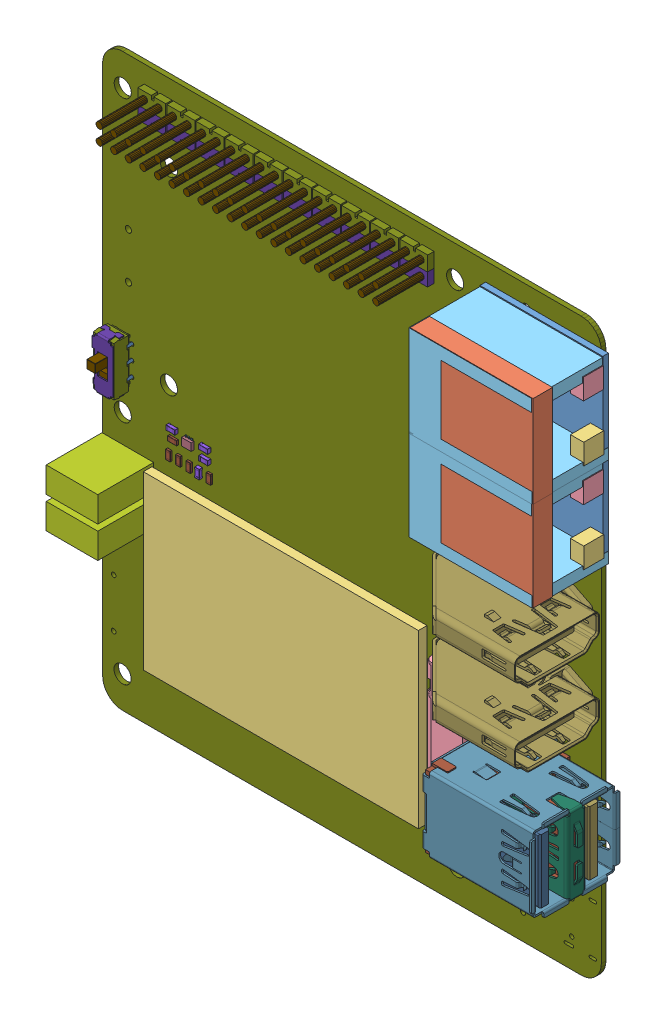
SolidWorks assembly CM4-DUAL-ETH-4G 5G-BASE, configuration Default. Lengths in mm. (continued)
Components (placement in the parent): (continued)
- CM4-DUAL-ETH-4G 5G-BASE.step-1: CM4-DUAL-ETH-4G 5G-BASE.step [Default] at origin size (91.94 99.62 20.53) (continued)
  - C51.step-1: C51.step [Default] at origin size (0.8 1.6 0.6)
    - CAPC1608(0603).step-1: CAPC1608(0603).step [Default] at (59.9278 -41.4202 -0.7984) x (0 1 0) z (0 0 -1) size (1.6 0.8 0.6)
  - C50.step-1: C50.step [Default] at origin size (1.6 0.8 0.6)
    - CAPC1608(0603).step-1: CAPC1608(0603).step [Default] at (29.923 -76.9062 0) x (1 0 0) z (0 0 1) size (1.6 0.8 0.6)
  - C49.step-1: C49.step [Default] at origin size (0.8 1.6 0.6)
    - CAPC1608(0603).step-1: CAPC1608(0603).step [Default] at (38.0407 -61.99 0) x (0 -1 0) z (0 0 1) size (1.6 0.8 0.6)
  - C48.step-1: C48.step [Default] at origin size (1.6 0.8 0.6)
    - CAPC1608(0603).step-1: CAPC1608(0603).step [Default] at (49.0658 -69.8064 0) x (-1 0 0) z (0 0 1) size (1.6 0.8 0.6)
  - C47.step-1: C47.step [Default] at origin size (0.8 1.6 0.6)
    - CAPC1608(0603).step-1: CAPC1608(0603).step [Default] at (39.4963 -61.99 0) x (0 -1 0) z (0 0 1) size (1.6 0.8 0.6)
  - C46.step-1: C46.step [Default] at origin size (1.6 0.8 0.6)
    - CAPC1608(0603).step-1: CAPC1608(0603).step [Default] at (49.0658 -71.2537 0) x (-1 0 0) z (0 0 1) size (1.6 0.8 0.6)
  - C44.step-1: C44.step [Default] at origin size (0.8 1.6 0.6)
    - CAPC1608(0603).step-1: CAPC1608(0603).step [Default] at (42.5195 -81.9688 -0.7984) x (0 1 0) z (0 0 -1) size (1.6 0.8 0.6)
  - C43.step-1: C43.step [Default] at origin size (1.6 0.8 0.6)
    - CAPC1608(0603).step-1: CAPC1608(0603).step [Default] at (49.1866 -62.69 0) x (-1 0 0) z (0 0 1) size (1.6 0.8 0.6)
  - C42.step-1: C42.step [Default] at origin size (1.6 0.8 0.6)
    - CAPC1608(0603).step-1: CAPC1608(0603).step [Default] at (49.0658 -74.1482 0) x (-1 0 0) z (0 0 1) size (1.6 0.8 0.6)
  - C41.step-1: C41.step [Default] at origin size (0.8 1.6 0.6)
    - CAPC1608(0603).step-1: CAPC1608(0603).step [Default] at (52.2225 -27.9219 -0.7984) x (0 1 0) z (0 0 -1) size (1.6 0.8 0.6)
  - C40.step-1: C40.step [Default] at origin size (1.6 0.8 0.6)
    - CAPC1608(0603).step-1: CAPC1608(0603).step [Default] at (49.1866 -63.8607 0) x (-1 0 0) z (0 0 1) size (1.6 0.8 0.6)
  - C39.step-1: C39.step [Default] at origin size (1.6 0.8 0.6)
    - CAPC1608(0603).step-1: CAPC1608(0603).step [Default] at (48.9722 -75.5798 0) x (-1 0 0) z (0 0 1) size (1.6 0.8 0.6)
  - C32.step-1: C32.step [Default] at origin size (1.6 0.8 0.6)
    - CAPC1608(0603).step-1: CAPC1608(0603).step [Default] at (51.5062 -32.7167 -0.7984) x (-1 0 0) z (0 0 -1) size (1.6 0.8 0.6)
  - C31.step-1: C31.step [Default] at origin size (0.8 1.6 0.6)
    - CAPC1608(0603).step-1: CAPC1608(0603).step [Default] at (48.8898 -27.9219 -0.7984) x (0 1 0) z (0 0 -1) size (1.6 0.8 0.6)
  - C30.step-1: C30.step [Default] at origin size (0.8 1.6 0.6)
    - CAPC1608(0603).step-1: CAPC1608(0603).step [Default] at (50.6641 -41.4202 -0.7984) x (0 1 0) z (0 0 -1) size (1.6 0.8 0.6)
  - C28.step-1: C28.step [Default] at origin size (0.8 1.6 0.6)
    - CAPC1608(0603).step-1: CAPC1608(0603).step [Default] at (53.758 -41.4202 -0.7984) x (0 1 0) z (0 0 -1) size (1.6 0.8 0.6)
  - C27.step-1: C27.step [Default] at origin size (0.8 1.6 0.6)
    - CAPC1608(0603).step-1: CAPC1608(0603).step [Default] at (52.2222 -41.4202 -0.7984) x (0 1 0) z (0 0 -1) size (1.6 0.8 0.6)
  - C26.step-1: C26.step [Default] at origin size (1.6 0.8 0.6)
    - CAPC1608(0603).step-1: CAPC1608(0603).step [Default] at (51.5325 -31.2588 -0.7984) x (1 0 0) z (0 0 -1) size (1.6 0.8 0.6)
  - C22.step-1: C22.step [Default] at origin size (1.6 0.8 0.6)
    - CAPC1608(0603).step-1: CAPC1608(0603).step [Default] at (51.5318 -35.5502 -0.7984) x (1 0 0) z (0 0 -1) size (1.6 0.8 0.6)
  - C21.step-1: C21.step [Default] at origin size (1.6 0.8 0.6)
    - CAPC1608(0603).step-1: CAPC1608(0603).step [Default] at (51.5318 -38.3867 -0.7984) x (1 0 0) z (0 0 -1) size (1.6 0.8 0.6)
  - C4.step-1: C4.step [Default] at origin size (0.8 1.6 0.6)
    - CAPC1608(0603).step-1: CAPC1608(0603).step [Default] at (56.9561 -77.7112 -0.7984) x (0 -1 0) z (0 0 -1) size (1.6 0.8 0.6)
  - C3.step-1: C3.step [Default] at origin size (1.27 2.72 0.46)
    - 663598576.step-1: 663598576.step [Default] at (56.9823 -82.7935 -1.2584) size (1.27 0.28 0.46)
      - Extruded-45.step-1: Extruded-45.step [Default] at origin size (1.27 0.28 0.46)
    - 663598576.step-2: 663598576.step [Default] at (56.9823 -80.3446 -1.2584) size (1.27 0.28 0.46)
      - Extruded-45.step-1: Extruded-45.step [Default] at origin size (1.27 0.28 0.46)
    - 764368928.step-1: 764368928.step [Default] at (56.9823 -81.6251 -1.2484) size (1.12 2.29 0.42)
      - Extruded-46.step-1: Extruded-46.step [Default] at origin size (1.12 2.29 0.42)
  - AMS-1.step-1: AMS-1.step [Default] at origin size (6.73 3.43 1.02)
    - 880594240.step-1: 880594240.step [Default] at (36.1772 -86.6648 0.254) size (6.73 3.43 1.02)
      - Extruded-47.step-1: Extruded-47.step [Default] at origin size (6.73 3.43 1.02)
  - R11.step-1: R11.step [Default] at origin size (0.8 1.6 0.38)
    - RESC1608(0603).step-1: RESC1608(0603).step [Default] at (64.5833 -30.5497 -0.7984) x (0 -1 0) z (1 0 0) size (1.6 0.38 0.8)
  - U3.step-1: U3.step [Default] at origin size (7.8 5.3 2.16)
    - 1503579216.step-1: 1503579216.step [Default] at (33.3767 -82.4828 -1.0524) size (1.3 0.41 0.25)
      - Extruded-48.step-1: Extruded-48.step [Default] at origin size (1.3 0.41 0.25)
    - 1503579216.step-2: 1503579216.step [Default] at (33.3767 -81.2128 -1.0524) size (1.3 0.41 0.25)
      - Extruded-48.step-1: Extruded-48.step [Default] at origin size (1.3 0.41 0.25)
    - 1503579216.step-3: 1503579216.step [Default] at (33.3767 -79.9428 -1.0524) size (1.3 0.41 0.25)
      - Extruded-48.step-1: Extruded-48.step [Default] at origin size (1.3 0.41 0.25)
    - 1503579216.step-4: 1503579216.step [Default] at (33.3767 -78.6728 -1.0524) size (1.3 0.41 0.25)
      - Extruded-48.step-1: Extruded-48.step [Default] at origin size (1.3 0.41 0.25)
    - 1503579216.step-5: 1503579216.step [Default] at (39.8767 -82.4928 -1.0524) size (1.3 0.41 0.25)
      - Extruded-48.step-1: Extruded-48.step [Default] at origin size (1.3 0.41 0.25)
    - 1503579216.step-6: 1503579216.step [Default] at (39.8767 -81.2228 -1.0524) size (1.3 0.41 0.25)
      - Extruded-48.step-1: Extruded-48.step [Default] at origin size (1.3 0.41 0.25)
    - 1503579216.step-7: 1503579216.step [Default] at (39.8767 -79.9528 -1.0524) size (1.3 0.41 0.25)
      - Extruded-48.step-1: Extruded-48.step [Default] at origin size (1.3 0.41 0.25)
    - 1503579216.step-8: 1503579216.step [Default] at (39.8767 -78.6828 -1.0524) size (1.3 0.41 0.25)
      - Extruded-48.step-1: Extruded-48.step [Default] at origin size (1.3 0.41 0.25)
    - 1503581520.step-1: 1503581520.step [Default] at (36.6267 -80.5828 -2.9584) size (5.4 5.3 2.01)
      - Extruded-49.step-1: Extruded-49.step [Default] at origin size (5.4 5.3 2.01)
  - R18.step-1: R18.step [Default] at origin size (0.8 1.6 0.38)
    - RESC1608(0603).step-1: RESC1608(0603).step [Default] at (36.3808 -80.8002 0) x (0 -1 0) z (-1 0 0) size (1.6 0.38 0.8)
  - R17.step-1: R17.step [Default] at origin size (1.6 0.8 0.38)
    - RESC1608(0603).step-1: RESC1608(0603).step [Default] at (29.8754 -75.3761 0) x (-1 0 0) z (0 1 0) size (1.6 0.38 0.8)
  - R16.step-1: R16.step [Default] at origin size (0.8 1.6 0.38)
    - RESC1608(0603).step-1: RESC1608(0603).step [Default] at (30.3209 -79.2715 -0.7984) x (0 -1 0) z (1 0 0) size (1.6 0.38 0.8)
  - R15.step-1: R15.step [Default] at origin size (0.8 1.6 0.38)
    - RESC1608(0603).step-1: RESC1608(0603).step [Default] at (50.6744 -27.9001 -0.7984) x (0 1 0) z (-1 0 0) size (1.6 0.38 0.8)
  - U4.step-1: U4.step [Default] at origin size (2.7 2.7 0.45)
    - 880596160.step-1: 880596160.step [Default] at (49.7296 -17.227 -1.2984) size (2.7 2.7 0.45)
      - Extruded-50.step-1: Extruded-50.step [Default] at origin size (2.7 2.7 0.45)
  - U5.step-1: U5.step [Default] at origin size (2 2.1 0.95)
    - User_Library-SC70-5-1.step-1: User_Library-SC70-5-1.step [Default] at (52.8539 -17.1936 -0.7984) x (1 0 0) z (0 0 -1) size (2 2.1 0.95)
  - R35.step-1: R35.step [Default] at origin size (0.8 1.6 0.38)
    - RESC1608(0603).step-1: RESC1608(0603).step [Default] at (52.2527 -11.5783 -0.7984) x (0 1 0) z (-1 0 0) size (1.6 0.38 0.8)
  - R33.step-1: R33.step [Default] at origin size (0.8 1.6 0.38)
    - RESC1608(0603).step-1: RESC1608(0603).step [Default] at (53.7884 -11.5783 -0.7984) x (0 1 0) z (-1 0 0) size (1.6 0.38 0.8)
  - D6.step-1: D6.step [Default] at origin size (1.35 2.6 1.14)
    - SW3dPS-SOD-323.step-1: SW3dPS-SOD-323.step [Default] at (51.0946 -21.502 -0.7984) x (0 -1 0) z (0 0 -1) size (2.6 1.35 1.14)
  - D5.step-1: D5.step [Default] at origin size (1.35 2.6 1.14)
    - SW3dPS-SOD-323.step-1: SW3dPS-SOD-323.step [Default] at (53.3476 -21.502 -0.7984) x (0 -1 0) z (0 0 -1) size (2.6 1.35 1.14)
  - C134.step-1: C134.step [Default] at origin size (0.8 1.6 0.6)
    - CAPC1608(0603).step-1: CAPC1608(0603).step [Default] at (55.1652 -21.3602 -0.7984) x (0 1 0) z (0 0 -1) size (1.6 0.8 0.6)
  - C133.step-1: C133.step [Default] at origin size (0.8 1.6 0.6)
    - CAPC1608(0603).step-1: CAPC1608(0603).step [Default] at (49.1745 -21.3865 -0.7984) x (0 -1 0) z (0 0 -1) size (1.6 0.8 0.6)
  - C38.step-1: C38.step [Default] at origin size (1.6 0.8 0.6)
    - CAPC1608(0603).step-1: CAPC1608(0603).step [Default] at (54.6319 -14.1546 -0.7984) x (1 0 0) z (0 0 -1) size (1.6 0.8 0.6)
  - C37.step-1: C37.step [Default] at origin size (0.8 1.6 0.6)
    - CAPC1608(0603).step-1: CAPC1608(0603).step [Default] at (55.1653 -17.2646 -0.7984) x (0 1 0) z (0 0 -1) size (1.6 0.8 0.6)
  - C36.step-1: C36.step [Default] at origin size (0.8 1.6 0.6)
    - CAPC1608(0603).step-1: CAPC1608(0603).step [Default] at (50.7103 -11.6263 -0.7984) x (0 -1 0) z (0 0 -1) size (1.6 0.8 0.6)
  - C35.step-1: C35.step [Default] at origin size (0.8 1.6 0.6)
    - CAPC1608(0603).step-1: CAPC1608(0603).step [Default] at (49.1745 -11.6263 -0.7984) x (0 -1 0) z (0 0 -1) size (1.6 0.8 0.6)
  - C9.step-1: C9.step [Default] at origin size (0.8 1.6 0.6)
    - CAPC1608(0603).step-1: CAPC1608(0603).step [Default] at (17.7596 -11.9503 -0.7984) x (0 1 0) z (0 0 -1) size (1.6 0.8 0.6)
  - C14.step-1: C14.step [Default] at origin size (0.8 1.6 0.6)
    - CAPC1608(0603).step-1: CAPC1608(0603).step [Default] at (77.2667 -94.9453 -0.7984) x (0 -1 0) z (0 0 -1) size (1.6 0.8 0.6)
  - C1.step-1: C1.step [Default] at origin size (0.8 1.6 0.6)
    - CAPC1608(0603).step-1: CAPC1608(0603).step [Default] at (39.7941 -94.4916 -0.7984) x (0 -1 0) z (0 0 -1) size (1.6 0.8 0.6)
  - U15.step-1: U15.step [Default] at origin size (2.5 3 1.1)
    - SW3DPS-SOT-23-5-DEFAULT.step-1: SW3DPS-SOT-23-5-DEFAULT.step [Default] at (9.4742 -18.2293 -1.2984) x (0 1 0) z (-1 0 0) size (3 1.1 2.5)
  - U12.step-1: U12.step [Default] at origin size (1.01 2.5 0.55)
    - User_Library-UDFN10.step-1: User_Library-UDFN10.step [Default] at (62.7073 -10.1236 0.1516) x (0 -1 0) z (1 0 0) size (2.5 0.55 1.01)
      - Body.step-1: Body.step [Default] at (1.0785 0.9721 1.8983) size (2.5 0.5 1)
      - Pin1.step-1: Pin1.step [Default] at (0.0785 1.0521 2.2208) x (0 0 -1) z (-1 0 0) size (0.36 0.13 0.2)
      - Pin2.step-1: Pin2.step [Default] at (0.5785 1.0521 2.2208) x (0 0 1) z (1 0 0) size (0.36 0.13 0.2)
      - Pin4.step-1: Pin4.step [Default] at (1.0785 0.9221 2.2208) x (0 0 1) z (-1 0 0) size (0.49 0.13 0.4)
      - Pin2.step-2: Pin2.step [Default] at (1.5785 0.9221 2.2208) x (0 0 1) z (-1 0 0) size (0.36 0.13 0.2)
      - Pin2.step-3: Pin2.step [Default] at (2.0785 0.9221 2.2208) x (0 0 1) z (-1 0 0) size (0.36 0.13 0.2)
      - Pin2.step-4: Pin2.step [Default] at (2.0785 0.9221 1.5758) x (0 0 -1) z (1 0 0) size (0.36 0.13 0.2)
      - Pin2.step-5: Pin2.step [Default] at (1.5785 0.9221 1.5758) x (0 0 -1) z (1 0 0) size (0.36 0.13 0.2)
      - Pin3.step-1: Pin3.step [Default] at (1.0785 0.9221 1.5758) x (0 0 1) z (-1 0 0) size (0.36 0.13 0.4)
      - Pin2.step-6: Pin2.step [Default] at (0.5785 0.9221 1.5758) x (0 0 -1) z (1 0 0) size (0.36 0.13 0.2)
      - Pin2.step-7: Pin2.step [Default] at (0.0785 0.9221 1.5758) x (0 0 -1) z (1 0 0) size (0.36 0.13 0.2)
  - U11.step-1: U11.step [Default] at origin size (2.5 3 1.1)
    - SW3DPS-SOT-23-5-DEFAULT.step-1: SW3DPS-SOT-23-5-DEFAULT.step [Default] at (50.4006 -45.1237 -1.2984) x (0 -1 0) z (1 0 0) size (3 1.1 2.5)
  - U9.step-1: U9.step [Default] at origin size (1.01 2.5 0.55)
    - User_Library-UDFN10.step-1: User_Library-UDFN10.step [Default] at (66.4724 -18.6329 0.1516) x (0 1 0) z (-1 0 0) size (2.5 0.55 1.01)
      - Body.step-1: Body.step [Default] at (1.0785 0.9721 1.8983) size (2.5 0.5 1)
      - Pin1.step-1: Pin1.step [Default] at (0.0785 1.0521 2.2208) x (0 0 -1) z (-1 0 0) size (0.36 0.13 0.2)
      - Pin2.step-1: Pin2.step [Default] at (0.5785 1.0521 2.2208) x (0 0 1) z (1 0 0) size (0.36 0.13 0.2)
      - Pin4.step-1: Pin4.step [Default] at (1.0785 0.9221 2.2208) x (0 0 1) z (-1 0 0) size (0.49 0.13 0.4)
      - Pin2.step-2: Pin2.step [Default] at (1.5785 0.9221 2.2208) x (0 0 1) z (-1 0 0) size (0.36 0.13 0.2)
      - Pin2.step-3: Pin2.step [Default] at (2.0785 0.9221 2.2208) x (0 0 1) z (-1 0 0) size (0.36 0.13 0.2)
      - Pin2.step-4: Pin2.step [Default] at (2.0785 0.9221 1.5758) x (0 0 -1) z (1 0 0) size (0.36 0.13 0.2)
      - Pin2.step-5: Pin2.step [Default] at (1.5785 0.9221 1.5758) x (0 0 -1) z (1 0 0) size (0.36 0.13 0.2)
      - Pin3.step-1: Pin3.step [Default] at (1.0785 0.9221 1.5758) x (0 0 1) z (-1 0 0) size (0.36 0.13 0.4)
      - Pin2.step-6: Pin2.step [Default] at (0.5785 0.9221 1.5758) x (0 0 -1) z (1 0 0) size (0.36 0.13 0.2)
      - Pin2.step-7: Pin2.step [Default] at (0.0785 0.9221 1.5758) x (0 0 -1) z (1 0 0) size (0.36 0.13 0.2)
  - R64.step-1: R64.step [Default] at origin size (0.8 1.6 0.38)
    - RESC1608(0603).step-1: RESC1608(0603).step [Default] at (12.5285 -18.2821 -0.7984) x (0 -1 0) z (1 0 0) size (1.6 0.38 0.8)
  - R57.step-1: R57.step [Default] at origin size (1.6 0.8 0.38)
    - RESC1608(0603).step-1: RESC1608(0603).step [Default] at (10.7955 -85.6126 0) x (-1 0 0) z (0 1 0) size (1.6 0.38 0.8)
  - R56.step-1: R56.step [Default] at origin size (1.6 0.8 0.38)
    - RESC1608(0603).step-1: RESC1608(0603).step [Default] at (10.8653 -83.8424 0) x (1 0 0) z (0 -1 0) size (1.6 0.38 0.8)
  - R55.step-1: R55.step [Default] at origin size (0.8 1.6 0.38)
    - RESC1608(0603).step-1: RESC1608(0603).step [Default] at (15.5482 -18.2821 -0.7984) x (0 -1 0) z (1 0 0) size (1.6 0.38 0.8)
  - R47.step-1: R47.step [Default] at origin size (0.8 1.6 0.38)
    - RESC1608(0603).step-1: RESC1608(0603).step [Default] at (55.3094 -11.6398 -0.7984) x (0 -1 0) z (1 0 0) size (1.6 0.38 0.8)
  - R46.step-1: R46.step [Default] at origin size (0.8 1.6 0.38)
    - RESC1608(0603).step-1: RESC1608(0603).step [Default] at (64.5833 -21.1257 -0.7984) x (0 -1 0) z (1 0 0) size (1.6 0.38 0.8)
  - R44.step-1: R44.step [Default] at origin size (0.8 1.6 0.38)
    - RESC1608(0603).step-1: RESC1608(0603).step [Default] at (19.5056 -11.9983 -0.7984) x (0 -1 0) z (1 0 0) size (1.6 0.38 0.8)
  - C84.step-1: C84.step [Default] at origin size (0.8 1.6 0.6)
    - CAPC1608(0603).step-1: CAPC1608(0603).step [Default] at (53.3602 -45.0643 -0.7984) x (0 -1 0) z (0 0 -1) size (1.6 0.8 0.6)
  - C83.step-1: C83.step [Default] at origin size (0.8 1.6 0.6)
    - CAPC1608(0603).step-1: CAPC1608(0603).step [Default] at (48.8898 -41.5988 -0.7984) x (0 -1 0) z (0 0 -1) size (1.6 0.8 0.6)
  - C82.step-1: C82.step [Default] at origin size (0.8 1.6 0.6)
    - CAPC1608(0603).step-1: CAPC1608(0603).step [Default] at (5.0212 -18.2595 -0.7984) x (0 -1 0) z (0 0 -1) size (1.6 0.8 0.6)
  - C79.step-1: C79.step [Default] at origin size (0.8 1.6 0.6)
    - CAPC1608(0603).step-1: CAPC1608(0603).step [Default] at (64.5899 -14.3235 -0.7984) x (0 1 0) z (0 0 -1) size (1.6 0.8 0.6)
  - C75.step-1: C75.step [Default] at origin size (0.8 1.6 0.6)
    - CAPC1608(0603).step-1: CAPC1608(0603).step [Default] at (6.5827 -18.234 -0.7984) x (0 1 0) z (0 0 -1) size (1.6 0.8 0.6)
  - C74.step-1: C74.step [Default] at origin size (0.8 1.6 0.6)
    - CAPC1608(0603).step-1: CAPC1608(0603).step [Default] at (14.0516 -18.2603 -0.7984) x (0 -1 0) z (0 0 -1) size (1.6 0.8 0.6)
  - C10.step-1: C10.step [Default] at origin size (0.8 1.6 0.6)
    - CAPC1608(0603).step-1: CAPC1608(0603).step [Default] at (50.1741 -81.8813 -0.7984) x (0 -1 0) z (0 0 -1) size (1.6 0.8 0.6)
  - C11.step-1: C11.step [Default] at origin size (0.8 1.6 0.6)
    - CAPC1608(0603).step-1: CAPC1608(0603).step [Default] at (48.3709 -81.855 -0.7984) x (0 1 0) z (0 0 -1) size (1.6 0.8 0.6)
  - C15.step-1: C15.step [Default] at origin size (0.8 1.6 0.6)
    - CAPC1608(0603).step-1: CAPC1608(0603).step [Default] at (59.8371 -27.9482 -0.7984) x (0 -1 0) z (0 0 -1) size (1.6 0.8 0.6)
  - C16.step-1: C16.step [Default] at origin size (1.6 0.8 0.6)
    - CAPC1608(0603).step-1: CAPC1608(0603).step [Default] at (51.5318 -36.9668 -0.7984) x (1 0 0) z (0 0 -1) size (1.6 0.8 0.6)
  - R8.step-1: R8.step [Default] at origin size (1.6 0.8 0.38)
    - RESC1608(0603).step-1: RESC1608(0603).step [Default] at (29.9452 -70.3512 0) x (1 0 0) z (0 -1 0) size (1.6 0.38 0.8)
  - R10.step-1: R10.step [Default] at origin size (0.8 1.6 0.38)
    - RESC1608(0603).step-1: RESC1608(0603).step [Default] at (42.5007 -79.0493 -0.7984) x (0 1 0) z (-1 0 0) size (1.6 0.38 0.8)
  - R12.step-1: R12.step [Default] at origin size (0.8 1.6 0.38)
    - RESC1608(0603).step-1: RESC1608(0603).step [Default] at (64.5936 -24.0283 -0.7984) x (0 1 0) z (-1 0 0) size (1.6 0.38 0.8)
  - U1.step-1: U1.step [Default] at origin size (2.5 3 1.1)
    - SW3DPS-SOT-23-5-DEFAULT.step-1: SW3DPS-SOT-23-5-DEFAULT.step [Default] at (53.5777 -77.8952 -1.2984) x (0 -1 0) z (1 0 0) size (3 1.1 2.5)
  - C19.step-1: C19.step [Default] at origin size (0.8 1.6 0.6)
    - CAPC1608(0603).step-1: CAPC1608(0603).step [Default] at (61.4628 -41.4202 -0.7984) x (0 1 0) z (0 0 -1) size (1.6 0.8 0.6)
  - TF1.step-1: TF1.step [Default] at origin size (13.82 14.45 2.1)
    - 1103521424.step-1: 1103521424.step [Default] at (7.383 -29.5195 -2.8984) size (13.82 14.45 0.1)
      - Extruded-51.step-1: Extruded-51.step [Default] at origin size (13.82 14.45 0.1)
    - 1103521296.step-1: 1103521296.step [Default] at (7.383 -29.5195 -2.8984) size (13.82 14.45 2.1)
      - Extruded-52.step-1: Extruded-52.step [Default] at origin size (13.82 14.45 2.1)
    - 1103521168.step-1: 1103521168.step [Default] at (7.383 -29.5195 -1.2984) size (13.82 14.45 0.5)
      - Extruded-53.step-1: Extruded-53.step [Default] at origin size (13.82 14.45 0.5)
  - CM-R1.step-1: CM-R1.step [Default] at origin size (0.85 1.65 0.46)
    - 575262224.step-1: 575262224.step [Default] at (42.7492 -93.7926 -1.2584) size (0.85 0.28 0.46)
      - Extruded-54.step-1: Extruded-54.step [Default] at origin size (0.85 0.28 0.46)
    - 575262224.step-2: 575262224.step [Default] at (42.7492 -95.1642 -1.2584) size (0.85 0.28 0.46)
      - Extruded-54.step-1: Extruded-54.step [Default] at origin size (0.85 0.28 0.46)
    - 575262352.step-1: 575262352.step [Default] at (42.7492 -94.4784 -1.2484) size (0.8 1.5 0.42)
      - Extruded-55.step-1: Extruded-55.step [Default] at origin size (0.8 1.5 0.42)
  - CM-R4.step-1: CM-R4.step [Default] at origin size (0.85 1.65 0.46)
    - 575262224.step-1: 575262224.step [Default] at (41.2717 -93.7926 -1.2584) size (0.85 0.28 0.46)
      - Extruded-54.step-1: Extruded-54.step [Default] at origin size (0.85 0.28 0.46)
    - 575262224.step-2: 575262224.step [Default] at (41.2717 -95.1642 -1.2584) size (0.85 0.28 0.46)
      - Extruded-54.step-1: Extruded-54.step [Default] at origin size (0.85 0.28 0.46)
    - 575262352.step-1: 575262352.step [Default] at (41.2717 -94.4784 -1.2484) size (0.8 1.5 0.42)
      - Extruded-55.step-1: Extruded-55.step [Default] at origin size (0.8 1.5 0.42)
  - L1.step-1: L1.step [Default] at origin size (9.95 4.45 11.5)
    - 1015527952.step-1: 1015527952.step [Default] at (7.7605 -62.6584 -1.5) x (0 1 0) z (0 0 1) size (0.76 0.76 5)
      - Cylinder.step-1: Cylinder.step [Default] at origin size (0.76 0.76 5)
    - 1015527952.step-2: 1015527952.step [Default] at (5.2205 -62.6584 -1.5) x (0 1 0) z (0 0 1) size (0.76 0.76 5)
      - Cylinder.step-1: Cylinder.step [Default] at origin size (0.76 0.76 5)
    - 1015527952.step-3: 1015527952.step [Default] at (5.2205 -60.1183 -1.5) x (0 1 0) z (0 0 1) size (0.76 0.76 5)
      - Cylinder.step-1: Cylinder.step [Default] at origin size (0.76 0.76 5)
    - 1015527952.step-4: 1015527952.step [Default] at (7.7605 -60.1183 -1.5) x (0 1 0) z (0 0 1) size (0.76 0.76 5)
      - Cylinder.step-1: Cylinder.step [Default] at origin size (0.76 0.76 5)
    - 1015527832.step-1: 1015527832.step [Default] at (0.9405 -61.3885 8) x (0 -1 0) z (0 0 1) size (3.5 3.5 3.5)
      - Sphere-13.step-1: Sphere-13.step [Default] at origin size (3.5 3.5 3.5)
    - 1103520528.step-1: 1103520528.step [Default] at (4.6411 -61.3877 0.254) size (9 4.45 9.75)
      - Extruded-12.step-1: Extruded-12.step [Default] at origin size (9 4.45 9.75)
    - 1015527712.step-1: 1015527712.step [Default] at (0.9405 -61.3885 3) x (0 -1 0) z (0 0 1) size (3.5 3.5 3.5)
      - Sphere.step-1: Sphere.step [Default] at origin size (3.5 3.5 3.5)
  - C45.step-1: C45.step [Default] at origin size (0.8 1.6 0.6)
    - CAPC1608(0603).step-1: CAPC1608(0603).step [Default] at (58.2116 -27.9482 -0.7984) x (0 -1 0) z (0 0 -1) size (1.6 0.8 0.6)
  - C12.step-1: C12.step [Default] at origin size (1.6 0.8 0.6)
    - CAPC1608(0603).step-1: CAPC1608(0603).step [Default] at (11.4515 -63.7998 -0.7984) x (1 0 0) z (0 0 -1) size (1.6 0.8 0.6)
  - C13.step-1: C13.step [Default] at origin size (1.6 0.8 0.6)
    - CAPC1608(0603).step-1: CAPC1608(0603).step [Default] at (16.0523 -67.4574 -0.7984) x (-1 0 0) z (0 0 -1) size (1.6 0.8 0.6)
  - Q5.step-1: Q5.step [Default] at origin size (2.64 3 1.08)
    - ALSRobot-SOT23.step-1: ALSRobot-SOT23.step [Default] at (17.3302 -60.1735 -0.7984) x (0 -1 0) z (0 0 -1) size (3 2.64 1.08)
  - R21.step-1: R21.step [Default] at origin size (1.6 0.8 0.38)
    - RESC1608(0603).step-1: RESC1608(0603).step [Default] at (11.4034 -65.5434 -0.7984) x (-1 0 0) z (0 -1 0) size (1.6 0.38 0.8)
  - R45.step-1: R45.step [Default] at origin size (1.6 0.8 0.38)
    - RESC1608(0603).step-1: RESC1608(0603).step [Default] at (20.7078 -63.8076 -0.7984) x (-1 0 0) z (0 -1 0) size (1.6 0.38 0.8)
  - R48.step-1: R48.step [Default] at origin size (1.6 3.2 0.6)
    - User_Library-CR3216-1206.step-1: User_Library-CR3216-1206.step [Default] at (21.1402 -59.9705 -0.7984) x (0 -1 0) z (1 0 0) size (3.2 0.6 1.6)
  - R49.step-1: R49.step [Default] at origin size (1.6 0.8 0.38)
    - RESC1608(0603).step-1: RESC1608(0603).step [Default] at (20.7776 -67.2557 -0.7984) x (1 0 0) z (0 1 0) size (1.6 0.38 0.8)
  - U2.step-1: U2.step [Default] at origin size (1.19 2.9 1.14)
    - 880594496.step-1: 880594496.step [Default] at (16.073 -64.5424 -1.9414) size (1.19 2.9 1.14)
      - Extruded-56.step-1: Extruded-56.step [Default] at origin size (1.19 2.9 1.14)
  - R74.step-1: R74.step [Default] at origin size (1.6 0.8 0.38)
    - RESC1608(0603).step-1: RESC1608(0603).step [Default] at (84.1244 -89.9694 -0.7984) x (1 0 0) z (0 1 0) size (1.6 0.38 0.8)
  - R75.step-1: R75.step [Default] at origin size (1.6 0.8 0.38)
    - RESC1608(0603).step-1: RESC1608(0603).step [Default] at (84.1244 -92.9694 -0.7984) x (1 0 0) z (0 1 0) size (1.6 0.38 0.8)
  - C103.step-1: C103.step [Default] at origin size (0.8 1.6 0.6)
    - CAPC1608(0603).step-1: CAPC1608(0603).step [Default] at (63.7716 -88.7373 -0.7984) x (0 -1 0) z (0 0 -1) size (1.6 0.8 0.6)
  - C104.step-1: C104.step [Default] at origin size (0.85 1.65 0.46)
    - 575262352.step-1: 575262352.step [Default] at (77.2669 -91.76 -1.2484) size (0.8 1.5 0.42)
      - Extruded-55.step-1: Extruded-55.step [Default] at origin size (0.8 1.5 0.42)
    - 575262224.step-1: 575262224.step [Default] at (77.2669 -92.4458 -1.2584) size (0.85 0.28 0.46)
      - Extruded-54.step-1: Extruded-54.step [Default] at origin size (0.85 0.28 0.46)
    - 575262224.step-2: 575262224.step [Default] at (77.2669 -91.0743 -1.2584) size (0.85 0.28 0.46)
      - Extruded-54.step-1: Extruded-54.step [Default] at origin size (0.85 0.28 0.46)
  - C105.step-1: C105.step [Default] at origin size (1.6 0.8 0.6)
    - CAPC1608(0603).step-1: CAPC1608(0603).step [Default] at (63.0809 -82.1182 -0.7984) x (-1 0 0) z (0 0 -1) size (1.6 0.8 0.6)
  - C106.step-1: C106.step [Default] at origin size (1.6 0.8 0.6)
    - CAPC1608(0603).step-1: CAPC1608(0603).step [Default] at (59.2175 -84.7976 -0.7984) x (1 0 0) z (0 0 -1) size (1.6 0.8 0.6)
  - C107.step-1: C107.step [Default] at origin size (1.65 0.85 0.46)
    - 575261968.step-1: 575261968.step [Default] at (68.0384 -80.896 -1.2484) size (1.5 0.8 0.42)
      - Extruded-4.step-1: Extruded-4.step [Default] at origin size (1.5 0.8 0.42)
    - 575262096.step-1: 575262096.step [Default] at (68.7242 -80.896 -1.2584) size (0.28 0.85 0.46)
      - Extruded-5.step-1: Extruded-5.step [Default] at origin size (0.28 0.85 0.46)
    - 575262096.step-2: 575262096.step [Default] at (67.3526 -80.896 -1.2584) size (0.28 0.85 0.46)
      - Extruded-5.step-1: Extruded-5.step [Default] at origin size (0.28 0.85 0.46)
  - C108.step-1: C108.step [Default] at origin size (1.6 0.8 0.6)
    - CAPC1608(0603).step-1: CAPC1608(0603).step [Default] at (68.0257 -79.3085 -0.7984) x (-1 0 0) z (0 0 -1) size (1.6 0.8 0.6)
  - R76.step-1: R76.step [Default] at origin size (0.8 1.6 0.38)
    - RESC1608(0603).step-1: RESC1608(0603).step [Default] at (61.9749 -88.6896 -0.7984) x (0 1 0) z (-1 0 0) size (1.6 0.38 0.8)
  - R77.step-1: R77.step [Default] at origin size (1.6 0.8 0.38)
    - RESC1608(0603).step-1: RESC1608(0603).step [Default] at (59.1749 -86.3098 -0.7984) x (-1 0 0) z (0 -1 0) size (1.6 0.38 0.8)
  - R79.step-1: R79.step [Default] at origin size (1.6 0.8 0.38)
    - RESC1608(0603).step-1: RESC1608(0603).step [Default] at (59.1749 -87.8287 -0.7984) x (-1 0 0) z (0 -1 0) size (1.6 0.38 0.8)
  - R80.step-1: R80.step [Default] at origin size (1.6 0.8 0.38)
    - RESC1608(0603).step-1: RESC1608(0603).step [Default] at (59.2447 -89.3608 -0.7984) x (1 0 0) z (0 1 0) size (1.6 0.38 0.8)
  - U16.step-1: U16.step [Default] at origin size (1.81 1.7 0.55)
    - 661965792.step-1: 661965792.step [Default] at (62.1545 -85.5846 -0.9584) size (0.4 0.23 0.16)
      - Extruded-57.step-1: Extruded-57.step [Default] at origin size (0.4 0.23 0.16)
    - 661965792.step-2: 661965792.step [Default] at (62.1545 -86.0845 -0.9584) size (0.4 0.23 0.16)
      - Extruded-57.step-1: Extruded-57.step [Default] at origin size (0.4 0.23 0.16)
    - 661965792.step-3: 661965792.step [Default] at (62.1545 -86.5845 -0.9584) size (0.4 0.23 0.16)
      - Extruded-57.step-1: Extruded-57.step [Default] at origin size (0.4 0.23 0.16)
    - 661965792.step-4: 661965792.step [Default] at (63.5565 -86.5846 -0.9584) size (0.4 0.23 0.16)
      - Extruded-57.step-1: Extruded-57.step [Default] at origin size (0.4 0.23 0.16)
    - 661965792.step-5: 661965792.step [Default] at (63.5565 -86.0846 -0.9584) size (0.4 0.23 0.16)
      - Extruded-57.step-1: Extruded-57.step [Default] at origin size (0.4 0.23 0.16)
    - 661965792.step-6: 661965792.step [Default] at (63.5565 -85.5846 -0.9584) size (0.4 0.23 0.16)
      - Extruded-57.step-1: Extruded-57.step [Default] at origin size (0.4 0.23 0.16)
    - 1348844112.step-1: 1348844112.step [Default] at (62.8544 -86.0846 -1.3484) size (1.3 1.7 0.5)
      - Extruded-58.step-1: Extruded-58.step [Default] at origin size (1.3 1.7 0.5)
  - C93.step-1: C93.step [Default] at origin size (1.6 0.8 0.6)
    - CAPC1608(0603).step-1: CAPC1608(0603).step [Default] at (14.7077 -83.849 0) x (1 0 0) z (0 0 1) size (1.6 0.8 0.6)
  - R6.step-1: R6.step [Default] at origin size (3.44 1.51 0.46)
    - 575262608.step-1: 575262608.step [Default] at (65.5642 -79.6989 -1.2584) size (0.28 1.51 0.46)
      - Extruded-59.step-1: Extruded-59.step [Default] at origin size (0.28 1.51 0.46)
    - 575262608.step-2: 575262608.step [Default] at (62.4017 -79.699 -1.2584) size (0.28 1.51 0.46)
      - Extruded-59.step-1: Extruded-59.step [Default] at origin size (0.28 1.51 0.46)
    - 1127966432.step-1: 1127966432.step [Default] at (63.9893 -79.7069 -1.2484) size (3.05 1.38 0.42)
      - Extruded-60.step-1: Extruded-60.step [Default] at origin size (3.05 1.38 0.42)
  - C87.step-1: C87.step [Default] at origin size (1.65 0.85 0.46)
    - 575261968.step-1: 575261968.step [Default] at (66.2355 -91.4092 -1.2484) size (1.5 0.8 0.42)
      - Extruded-4.step-1: Extruded-4.step [Default] at origin size (1.5 0.8 0.42)
    - 575262096.step-1: 575262096.step [Default] at (65.5498 -91.4092 -1.2584) size (0.28 0.85 0.46)
      - Extruded-5.step-1: Extruded-5.step [Default] at origin size (0.28 0.85 0.46)
    - 575262096.step-2: 575262096.step [Default] at (66.9213 -91.4092 -1.2584) size (0.28 0.85 0.46)
      - Extruded-5.step-1: Extruded-5.step [Default] at origin size (0.28 0.85 0.46)
  - U10.step-1: U10.step [Default] at origin size (4.94 3.1 1.1)
    - User_Library-MSOP8.step-1: User_Library-MSOP8.step [Default] at (68.0617 -93.7668 -1.8984) x (1 0 0) z (0 1 0) size (4.94 1.1 3.1)
  - C20.step-1: C20.step [Default] at origin size (1.6 0.8 0.6)
    - CAPC1608(0603).step-1: CAPC1608(0603).step [Default] at (11.4514 -67.2408 -0.7984) x (1 0 0) z (0 0 -1) size (1.6 0.8 0.6)
  - HDMI0.step-1: HDMI0.step [Default] at origin size (23.1 7.88 20.15)
    - 72r3759_2007435-1.step-1: 72r3759_2007435-1.step [Default] at (88.2992 -56.8507 9) x (0 1 0) z (1 0 0) size (7.88 20.15 23.1)
  - Board.step-1: Board.step [Default] at (0 0 -0.7984) size (87.02 99.62 0.8)
